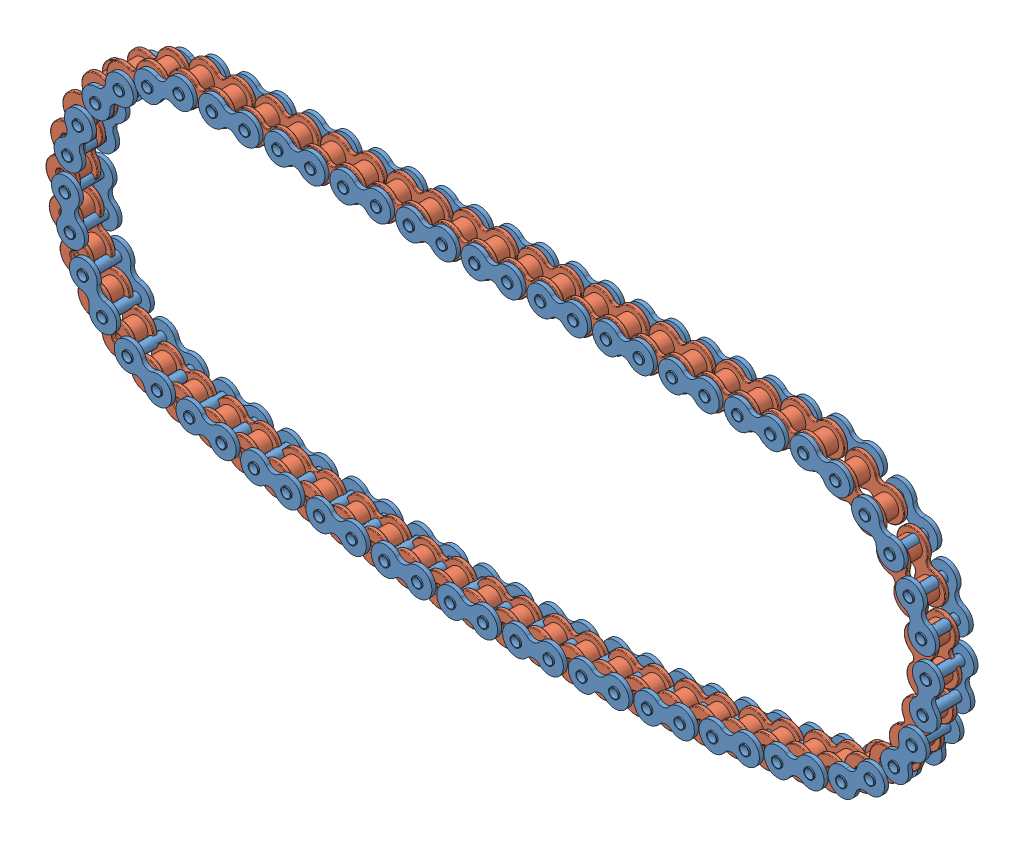
SolidWorks assembly Assem1, configuration Default. Lengths in mm.
Overall size (347.32 130.94 15.57).
2 component instances, 2 part files, 3 mates.
Components (placement in the parent):
- inner chain-1: inner chain [Default] at (50.8838 237.4417 295.2564) size (343.48 129.34 15.57)
- outer chain-1: outer chain [Default] at (63.5838 237.4539 285.7441) x (1 0.000147 0) z (0 0 1) size (344.76 130.89 9.51)
Mates (geometry in assembly coordinates):
- Concentric3: concentric aligned: cylinder of inner chain-1 through (-31.6662 237.4417 297.3519) axis (0 0 -1) radius 1.9812; cylinder of outer chain-1 through (-31.6662 237.4417 295.2564) axis (0 0 -1) radius 2.2352
- Concentric4: concentric aligned: cylinder of inner chain-1 through (-18.9662 237.4417 297.3519) axis (0 0 -1) radius 1.9812; cylinder of outer chain-1 through (-18.9662 237.4417 287.3316) axis (0 0 -1) radius 1.9812
- Coincident2: coincident anti-aligned: plane of inner chain-1 through (-46.5832 233.2128 295.2564) normal (0 0 -1); plane of outer chain-1 through (-44.3662 237.4361 295.2564) normal (0 0 1)
